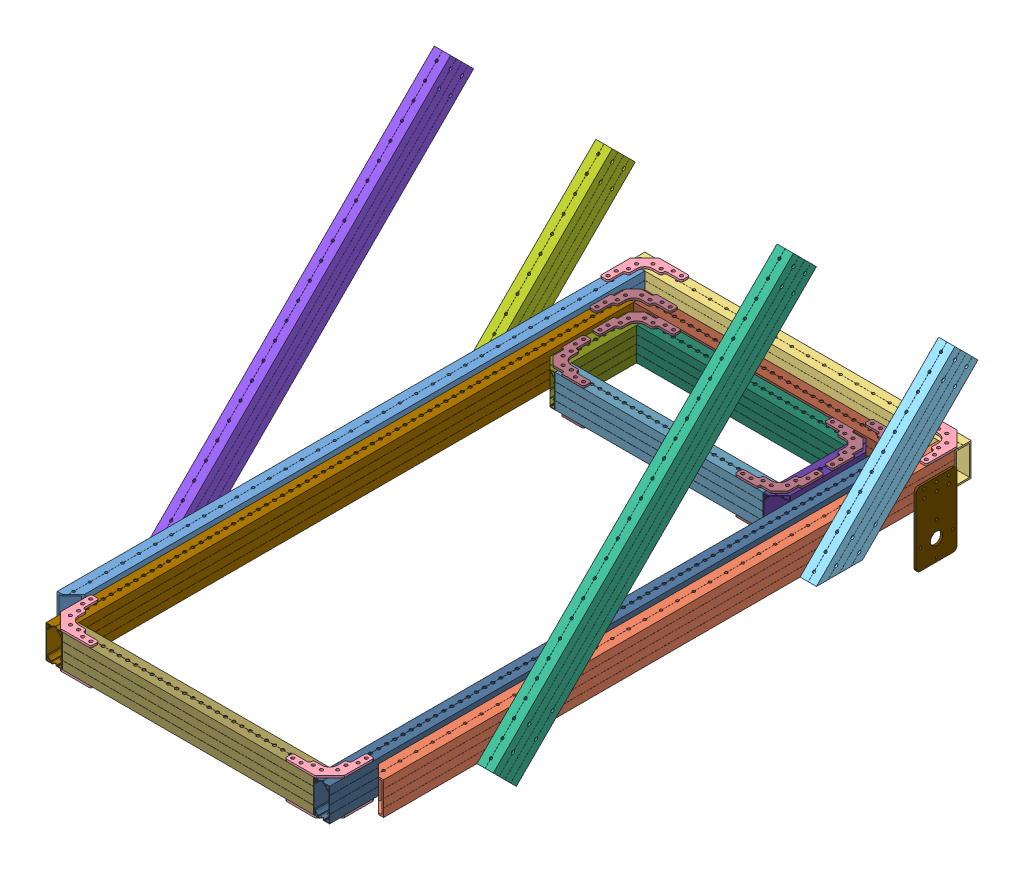
SolidWorks assembly 02-000 Elevator New, configuration Default. Lengths in mm.
Overall size (558.8 559.36 1000.52).
50 component instances, 18 part files, 21 mates.
Components (placement in the parent):
- 02-A-000 Elevator Frame New-1: 02-A-000 Elevator Frame New [Default] at origin size (558.8 502.89 917.1) (flexible)
  - 02-A-001 Elevator Frame Left Side-1: 02-A-001 Elevator Frame Left Side [Outer Side] at (-241.3 0 12.7) size (25.4 50.8 889)
  - 02-A-002 Elevator Frame Right Side-1: 02-A-002 Elevator Frame Right Side [Outer Side] at (241.3 0 12.7) size (25.4 50.8 889)
  - 02-A-003 Elevator Frame Bottom-1: 02-A-003 Elevator Frame Bottom [Outer Cross] at (12.7 0 -444.5) x (0 0 -1) z (1 0 0) size (25.4 50.8 508)
  - 2x1 Cam Follower Bearing Assembly-1: 2x1 Cam Follower Bearing Assembly [Default_speedpak] at (521.16 144.7702 66.2519) x (0 -1 0) z (-1 0 0) size (79.93 36.04 25.88)
  - 2x1 Cam Follower Bearing Assembly-2: 2x1 Cam Follower Bearing Assembly [Default_speedpak] at (-521.16 -144.7702 66.2519) x (0 1 0) z (1 0 0) size (79.93 36.04 25.88)
  - Elevator Corner Bracket-2: Elevator Corner Bracket [Default] at (254 -25.4 -457.2) x (0 0 1) z (1 0 0) size (69.85 3.17 69.85)
  - Elevator Corner Bracket-4: Elevator Corner Bracket [Default] at (-254 -28.575 -457.2) x (0 0 1) z (-1 0 0) size (69.85 3.17 69.85)
  - Elevator Corner Bracket-5: Elevator Corner Bracket [Default] at (254 28.575 -457.2) x (0 0 1) z (1 0 0) size (69.85 3.17 69.85)
  - Elevator Corner Bracket-6: Elevator Corner Bracket [Default] at (-254 25.4 -457.2) x (0 0 1) z (-1 0 0) size (69.85 3.17 69.85)
  - 02-A-004 Elevator Frame Tower Back Right-1: 02-A-004 Elevator Frame Tower Back Right [Outer Cross] at (266.7 73.3828 -325.5777) x (1 0 0) z (0 0.707107 -0.707107) size (25.4 50.8 304.8)
  - 02-A-005 Elevator Frame Tower Front Right-1: 02-A-005 Elevator Frame Tower Front Right [Tower Front] at (266.7 181.1459 69.5536) x (1 0 0) z (0 -0.707107 0.707107) size (25.4 50.8 660.4)
  - 02-A-006 Elevator Frame Tower Back Left-1: 02-A-006 Elevator Frame Tower Back Left [Outer Cross] at (-266.7 73.3828 -325.5777) x (1 0 0) z (0 0.707107 -0.707107) size (25.4 50.8 304.8)
  - 02-A-007 Elevator Frame Tower Front Left-1: 02-A-007 Elevator Frame Tower Front Left [Tower Front] at (-266.7 181.1459 69.5536) x (1 0 0) z (0 -0.707107 0.707107) size (25.4 50.8 660.4)
- 02-B-000 Elevator Stage 1 New-1: 02-B-000 Elevator Stage 1 New [Default] at (0 0 50.8) size (473.08 79.93 917.1)
  - 02-B-003 Elevator Stage Left Side-1: 02-B-003 Elevator Stage Left Side [Inner Length] at (-207.9625 0 596.9) size (25.4 50.8 914.4)
  - 02-B-004 Elevator Stage Right Side-1: 02-B-004 Elevator Stage Right Side [Inner Length] at (207.9625 0 596.9) size (25.4 50.8 914.4)
  - 02-B-002 Elevator Stage Bottom-1: 02-B-002 Elevator Stage Bottom [Inner Cross] at (566.7375 0 -444.5) x (0 0 -1) z (1 0 0) size (25.4 50.8 390.53)
  - 02-B-001 Elevator Stage Top-1: 02-B-001 Elevator Stage Top [Inner Cross] at (566.7375 0 444.5) x (0 0 -1) z (1 0 0) size (25.4 50.8 390.53)
  - 02-001 Elevator Corner Bracket with Bearing Cutout-1: 02-001 Elevator Corner Bracket with Bearing Cutout [Default] at (-220.6625 25.4 -457.2) x (0 0 1) z (-1 0 0) size (69.85 3.17 69.85)
  - 02-001 Elevator Corner Bracket with Bearing Cutout-2: 02-001 Elevator Corner Bracket with Bearing Cutout [Default] at (220.6625 25.4 -457.2) x (-1 0 0) z (0 0 -1) size (69.85 3.17 69.85)
  - Elevator Corner Bracket-10: Elevator Corner Bracket [Default] at (220.6625 25.4 457.2) x (0 0 -1) z (1 0 0) size (69.85 3.17 69.85)
  - Elevator Corner Bracket-9: Elevator Corner Bracket [Default] at (-220.6625 25.4 457.2) size (69.85 3.17 69.85)
  - 02-001 Elevator Corner Bracket with Bearing Cutout-5: 02-001 Elevator Corner Bracket with Bearing Cutout [Default] at (-220.6625 -28.575 -457.2) x (0 0 1) z (-1 0 0) size (69.85 3.17 69.85)
  - Elevator Corner Bracket-11: Elevator Corner Bracket [Default] at (-220.6625 -28.575 457.2) size (69.85 3.17 69.85)
  - Elevator Corner Bracket-12: Elevator Corner Bracket [Default] at (220.6625 -28.575 457.2) x (0 0 -1) z (1 0 0) size (69.85 3.17 69.85)
  - 02-001 Elevator Corner Bracket with Bearing Cutout-8: 02-001 Elevator Corner Bracket with Bearing Cutout [Default] at (220.6625 -28.575 -457.2) x (-1 0 0) z (0 0 -1) size (69.85 3.17 69.85)
  - 2x1 Cam Follower Bearing Assembly-1: 2x1 Cam Follower Bearing Assembly [Default_speedpak] at (71.8975 -144.7702 -66.2519) x (0 1 0) z (-1 0 0) size (79.93 36.04 25.88)
  - 2x1 Cam Follower Bearing Assembly-2: 2x1 Cam Follower Bearing Assembly [Default_speedpak] at (-71.8975 144.7702 -66.2519) x (0 -1 0) z (1 0 0) size (79.93 36.04 25.88)
- 02-C-000 Elevator Carriage-1: 02-C-000 Elevator Carriage [Default] at (0 0 -301.625) x (1 0 0) z (0 0 -1) size (406.4 79.93 157.8)
  - 02-C-001 Elevator Carriage Top-1: 02-C-001 Elevator Carriage Top [Carriage Cross] at (-574.675 0 -63.5) x (0 0 1) z (-1 0 0) size (25.4 50.8 323.85)
  - 02-C-002 Elevator Carriage Bottom-1: 02-C-002 Elevator Carriage Bottom [Carriage Cross] at (-574.675 0 63.5) x (0 0 1) z (-1 0 0) size (25.4 50.8 323.85)
  - 02-C-003 Elevator Carriage Left Side-1: 02-C-003 Elevator Carriage Left Side [Carriage Length] at (-174.625 0 584.2) size (25.4 50.8 152.4)
  - 02-C-004 Elevator Carriage Right Side-1: 02-C-004 Elevator Carriage Right Side [Carriage Length] at (174.625 0 584.2) size (25.4 50.8 152.4)
  - 02-001 Elevator Corner Bracket with Bearing Cutout-3: 02-001 Elevator Corner Bracket with Bearing Cutout [Default] at (-187.325 25.4 76.2) size (69.85 3.17 69.85)
  - 02-001 Elevator Corner Bracket with Bearing Cutout-2: 02-001 Elevator Corner Bracket with Bearing Cutout [Default] at (-187.325 25.4 -76.2) x (0 0 1) z (-1 0 0) size (69.85 3.17 69.85)
  - 02-001 Elevator Corner Bracket with Bearing Cutout-5: 02-001 Elevator Corner Bracket with Bearing Cutout [Default] at (187.325 25.4 76.2) x (0 0 -1) z (1 0 0) size (69.85 3.17 69.85)
  - 02-001 Elevator Corner Bracket with Bearing Cutout-4: 02-001 Elevator Corner Bracket with Bearing Cutout [Default] at (187.325 25.4 -76.2) x (-1 0 0) z (0 0 -1) size (69.85 3.17 69.85)
  - 2x1 Cam Follower Bearing Assembly-1: 2x1 Cam Follower Bearing Assembly [Default_speedpak] at (105.235 144.7702 -314.7481) x (0 -1 0) z (-1 0 0) size (79.93 36.04 25.88)
  - 02-001 Elevator Corner Bracket with Bearing Cutout-6: 02-001 Elevator Corner Bracket with Bearing Cutout [Default] at (-187.325 -28.575 76.2) size (69.85 3.17 69.85)
  - 02-001 Elevator Corner Bracket with Bearing Cutout-7: 02-001 Elevator Corner Bracket with Bearing Cutout [Default] at (187.325 -28.575 -76.2) x (-1 0 0) z (0 0 -1) size (69.85 3.17 69.85)
  - 02-001 Elevator Corner Bracket with Bearing Cutout-8: 02-001 Elevator Corner Bracket with Bearing Cutout [Default] at (187.325 -28.575 76.2) x (0 0 -1) z (1 0 0) size (69.85 3.17 69.85)
  - 02-001 Elevator Corner Bracket with Bearing Cutout-9: 02-001 Elevator Corner Bracket with Bearing Cutout [Default] at (-187.325 -28.575 -76.2) x (0 0 1) z (-1 0 0) size (69.85 3.17 69.85)
  - 2x1 Cam Follower Bearing Assembly-4: 2x1 Cam Follower Bearing Assembly [Default_speedpak] at (105.235 -144.7702 314.7481) x (0 1 0) z (-1 0 0) size (79.93 36.04 25.88)
  - 2x1 Cam Follower Bearing Assembly-5: 2x1 Cam Follower Bearing Assembly [Default_speedpak] at (-105.235 -144.7702 -314.7481) x (0 1 0) z (1 0 0) size (79.93 36.04 25.88)
  - 2x1 Cam Follower Bearing Assembly-6: 2x1 Cam Follower Bearing Assembly [Default_speedpak] at (-105.235 144.7702 314.7481) x (0 -1 0) z (1 0 0) size (79.93 36.04 25.88)
- MAXPlanetary 2-Stage NEO Example-1: MAXPlanetary 2-Stage NEO Example [Default_speedpak] at (228.6 -76.2 -314.325) x (0 -1 0) z (0 0 -1) size (89.61 89.51 122.08)
- MAX 90 Degree Gearbox (REV-21-2120)-1: MAX 90 Degree Gearbox (REV-21-2120) [Default_speedpak] at (228.6 -76.2 -381.3) x (0 -1 0) z (1 0 0) size (63.5 63.5 50.8)
- 02-002 Motor Mounting Bracket-1: 02-002 Motor Mounting Bracket [Default] at (254 6.35 -431.8) x (1 0 0) z (0 0 -1) size (3.17 114.3 63.5)
- MAXPlanetary 2-Stage NEO Example-2: MAXPlanetary 2-Stage NEO Example [Default_speedpak] at (104.775 -57.15 -444.5) x (0 0 1) z (-1 0 0) size (89.61 89.51 122.08)
Mates (geometry in assembly coordinates):
- Coincident1: coincident aligned: plane of 02-A-000 Elevator Frame New-1/02-A-003 Elevator Frame Bottom-1 through (762 25.4 -431.8) normal (0 1 0); plane of 02-B-000 Elevator Stage 1 New-1/02-B-002 Elevator Stage Bottom-1 through (-614.3625 25.4 -406.4) normal (0 1 0)
- Width1: width aligned: plane of 02-B-000 Elevator Stage 1 New-1/02-B-004 Elevator Stage Right Side-1 through (220.6625 -25.4 -533.4) normal (1 0 0); plane of 02-A-000 Elevator Frame New-1/02-A-001 Elevator Frame Left Side-1 through (-220.6625 -25.4 -533.4) normal (-1 0 0); plane of 02-B-000 Elevator Stage 1 New-1/02-B-003 Elevator Stage Left Side-1 through (-228.6 -25.4 762) normal (1 0 0); plane of 02-A-000 Elevator Frame New-1/02-A-002 Elevator Frame Right Side-1 through (228.6 -25.4 762) normal (-1 0 0)
- Coincident2: coincident aligned: plane of 02-B-000 Elevator Stage 1 New-1/02-B-002 Elevator Stage Bottom-1 through (-614.3625 25.4 -406.4) normal (0 1 0); plane of 02-C-000 Elevator Carriage-1/02-C-002 Elevator Carriage Bottom-1 through (606.425 25.4 -377.825) normal (0 1 0)
- Width2: width aligned: plane of 02-C-000 Elevator Carriage-1/02-C-003 Elevator Carriage Left Side-1 through (-187.325 25.4 295.275) normal (-1 0 0); plane of 02-B-000 Elevator Stage 1 New-1/02-B-004 Elevator Stage Right Side-1 through (187.325 25.4 295.275) normal (1 0 0); plane of 02-C-000 Elevator Carriage-1/02-C-004 Elevator Carriage Right Side-1 through (195.2625 -25.4 -533.4) normal (-1 0 0); plane of 02-B-000 Elevator Stage 1 New-1/02-B-003 Elevator Stage Left Side-1 through (-195.2625 -25.4 -533.4) normal (1 0 0)
- LimitDistance2: limit distance = 311.0896 mm anti-aligned: plane of 02-C-000 Elevator Carriage-1/02-C-002 Elevator Carriage Bottom-1 through (606.425 25.4 -377.825) normal (0 0 -1); plane of 02-B-000 Elevator Stage 1 New-1/02-B-002 Elevator Stage Bottom-1 through (-614.3625 -25.4 -381) normal (0 0 1)
- LimitDistance3: limit distance = 400.1104 mm anti-aligned: plane of 02-C-000 Elevator Carriage-1/02-C-001 Elevator Carriage Top-1 through (606.425 25.4 -225.425) normal (0 0 1); plane of 02-B-000 Elevator Stage 1 New-1/02-B-001 Elevator Stage Top-1 through (-614.3625 -25.4 482.6) normal (0 0 -1)
- Coincident3: coincident anti-aligned: plane of MAXPlanetary 2-Stage NEO Example-1 through (228.6 -76.2 -368.3) normal (0 0 -1); plane of MAX 90 Degree Gearbox (REV-21-2120)-1 through (228.6 -76.2 -368.3) normal (0 0 1)
- Concentric1: concentric aligned: circle of MAXPlanetary 2-Stage NEO Example-1; cylinder of MAX 90 Degree Gearbox (REV-21-2120)-1 through (228.6 -101.6 -368.3) axis (0 0 -1) radius 2.5
- Coincident4: coincident anti-aligned: plane of 02-A-000 Elevator Frame New-1/02-A-002 Elevator Frame Right Side-1 through (254 -25.4 762) normal (1 0 0); plane of 02-002 Motor Mounting Bracket-1 through (254 6.35 -431.8) normal (-1 0 0)
- Distance2: distance = 19.05 mm aligned: plane of 02-A-000 Elevator Frame New-1/02-A-002 Elevator Frame Right Side-1 through (228.6 25.4 762) normal (0 1 0); plane of 02-002 Motor Mounting Bracket-1 through (257.175 6.35 -431.8) normal (0 1 0)
- Coincident6: coincident anti-aligned: plane of MAX 90 Degree Gearbox (REV-21-2120)-1 through (254 -76.2 -400.05) normal (1 0 0); plane of 02-002 Motor Mounting Bracket-1 through (254 6.35 -431.8) normal (-1 0 0)
- Coincident7: coincident anti-aligned: plane of 02-A-000 Elevator Frame New-1/02-A-003 Elevator Frame Bottom-1 through (762 -25.4 -431.8) normal (0 0 1); plane of 02-002 Motor Mounting Bracket-1 through (257.175 6.35 -431.8) normal (0 0 -1)
- Coincident8: coincident aligned: plane of MAX 90 Degree Gearbox (REV-21-2120)-1 through (254 -107.95 -400.05) normal (0 -1 0); plane of 02-002 Motor Mounting Bracket-1 through (257.175 -107.95 -431.8) normal (0 -1 0)
- Concentric2: concentric aligned: circle of MAXPlanetary 2-Stage NEO Example-1; cylinder of MAX 90 Degree Gearbox (REV-21-2120)-1 through (228.6 -50.8 -368.3) axis (0 0 -1) radius 2.5
- Coincident9: coincident aligned: plane of MAX 90 Degree Gearbox (REV-21-2120)-1 through (254 -76.2 -431.8) normal (0 0 -1); plane of 02-002 Motor Mounting Bracket-1 through (257.175 6.35 -431.8) normal (0 0 -1)
- LimitDistance4: limit distance = 193.1174 mm anti-aligned: plane of 02-A-000 Elevator Frame New-1/02-A-003 Elevator Frame Bottom-1 through (762 -25.4 -431.8) normal (0 0 1); plane of 02-B-000 Elevator Stage 1 New-1/02-B-002 Elevator Stage Bottom-1 through (-614.3625 -25.4 -406.4) normal (0 0 -1)
- Symmetric3: symmetric aligned: plane of 02-C-000 Elevator Carriage-1/02-C-002 Elevator Carriage Bottom-1 through (606.425 25.4 -377.825) normal (0 0 -1)
- LimitDistance5: limit distance = 3.175 mm anti-aligned: plane of 02-B-000 Elevator Stage 1 New-1/02-B-002 Elevator Stage Bottom-1 through (-614.3625 -25.4 -381) normal (0 0 1); plane of 02-C-000 Elevator Carriage-1/02-C-002 Elevator Carriage Bottom-1 through (606.425 25.4 -377.825) normal (0 0 -1)
- Distance3: distance = 6.35 mm: plane of MAXPlanetary 2-Stage NEO Example-2 through (69.85 -31.75 -419.1) normal (0 1 0); plane of 02-A-000 Elevator Frame New-1/02-A-003 Elevator Frame Bottom-1 through (762 -25.4 -431.8) normal (0 -1 0)
- Concentric3: concentric: unknown of 02-A-000 Elevator Frame New-1/02-A-003 Elevator Frame Bottom-1; unknown of ?
- Parallel1: parallel aligned: plane of 02-A-000 Elevator Frame New-1/02-A-003 Elevator Frame Bottom-1 through (-254 0 -444.5) normal (-1 0 0); plane of ? through (50.8 -28.7525 -438.5878) normal (-1 0 0)
